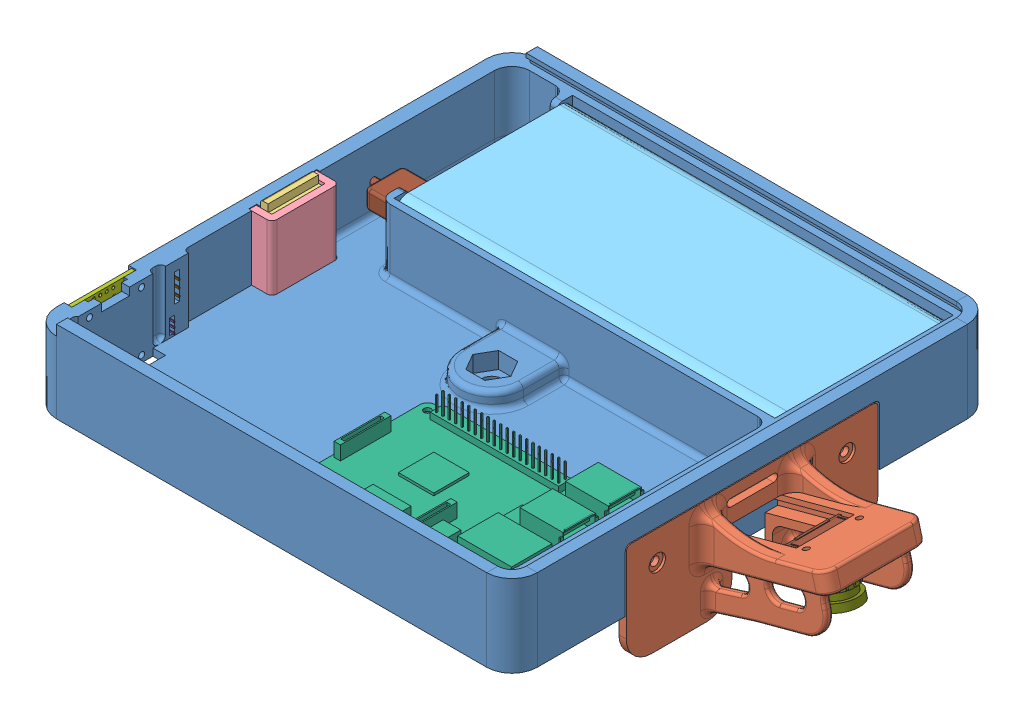
SolidWorks assembly vision, configuration Défaut. Lengths in mm.
Overall size (246.21 50.4 190).
58 component instances, 37 part files, 59 mates.
Components (placement in the parent):
- box-1: box [Défaut] at origin size (190.6 32.4 190)
- cover-1: cover [Défaut] at (-1.3 28.3 0) x (0 0 1) z (-1 0 0) size (190 2 187) (hidden)
- LogoARIG2-1: LogoARIG2 [Défaut] at (29.3179 30.3 42.8) x (0 0 -1) z (0 1 0) size (88.08 45.8 6.03) (hidden)
- support-cam-1: support-cam [Défaut] at (92 2.85 0) x (0 0 -1) z (1 0 0) size (99.5 41.7 53.04)
- latch-1: latch [Défaut] at (-84.4 7.063 -10) size (14.06 23.3 20)
- latch-box-1: latch-box [Défaut] at (-81.6 1.6 0) x (0 0 -1) z (1 0 0) size (26.6 26.5 9)
- Xiaomi PowerBank-1: Xiaomi PowerBank [Défaut] at (84.75 2.8 -89.15) x (0 0 1) z (-1 0 0) size (70 25 150)
- raspberryPi3BSimplified_STEP.step-1: raspberryPi3BSimplified_STEP.step [Défaut] at (32.5 6.8 51.4) x (1 0 0) z (0 1 0) size (87 58.5 18.55)
- OSSD-128x64.igs-1: OSSD-128x64.igs [Défaut] at (-91.9 15.3 69.5) x (0 0 1) z (0 -1 0) size (25 5.1 26)
- micro push button-2: micro push button [Défaut] at (-89.5 6.8667 45.1) x (0 -1 0) z (0 0 -1) size (5.8 13.4 5.8)
- mini swich-1: mini swich [Défaut] at (-89.9 19.2833 45.2) x (0 1 0) z (0 0 1) size (10.5 12.4 5.6)
- spring-1: spring [Défaut] at (-87.002 2.3106 6.0058) x (0.974863 -0.040201 -0.21915) z (0.219381 0.001367 0.975638) size (4.02 10.6 4.01)
- spring-2: spring [Défaut] at (-87.0662 11.9402 -5.894) x (-0.826432 0.000175 -0.563036) z (-0.56297 -0.015546 0.826331) size (4.02 10.6 4.01)
- usb-port-1: usb-port [Défaut] at (-65.85 15.3 -33.65) x (0 0 1) z (-1 0 0) size (15.2 7.3 34.7)
- RspCameraMia-1: RspCameraMia [Défaut] at (130.1784 16.2188 -0.0942) x (0.965926 0.258819 0) z (0.258819 -0.965926 0) size (23.86 25 22.7)
  - RspCameraMia.stp-1: RspCameraMia.stp [Défaut] at origin size (23.86 25 9.96)
    - 70521906.stp-1: 70521906.stp [Défaut] at (1.7167 0.8597 0.0159) size (2 2.1 0.95)
      - 70521906_01.stp-1: 70521906_01.stp [Défaut] at origin size (0.25 0.55 0.75)
      - 70521906_02.stp-1: 70521906_02.stp [Défaut] at origin size (0.25 0.55 0.75)
      - 70521906_03.stp-1: 70521906_03.stp [Défaut] at origin size (2 1.25 0.9)
      - 70521906_04.stp-1: 70521906_04.stp [Défaut] at origin size (0.25 0.55 0.75)
      - 70521906_05.stp-1: 70521906_05.stp [Défaut] at origin size (0.25 0.55 0.75)
      - 70521906_06.stp-1: 70521906_06.stp [Défaut] at origin size (0.25 0.55 0.75)
      - 70521906_07.stp-1: 70521906_07.stp [Défaut] at origin size (0.25 0.55 0.75)
    - PicameraPCB.stp-1: PicameraPCB.stp [Défaut] at (0.2393 -0.0199 0) x (-1 0 0) z (0 0 1) size (23.86 25 2.2)
    - OVA5647_Housing.stp-1: OVA5647_Housing.stp [Défaut] at (-2.4078 0.0859 1) x (1 0 0) z (0 -1 0) size (8 3.95 8)
    - OVA5647_Lens_FOV.stp-1: OVA5647_Lens_FOV.stp [Défaut] at (-2.4087 0.0921 5.963) x (1 0 0) z (0 -1 0) size (6 3.35 6)
    - ribbon_cam.stp-1: ribbon_cam.stp [Défaut] at (-2.4804 0.3633 1.4162) x (0 1 0) z (1 0 0) size (5.6 0.69 4.76)
    - CCD.stp-1: CCD.stp [Défaut] at (-2.0757 0.287 1.296) x (1 0 0) z (0 -1 0) size (8.01 0.69 8.01)
    - CAPC-0805-T0.75-BN.stp-1: CAPC-0805-T0.75-BN.stp [Défaut] at (4.562 5.9833 -0.0026) x (0 -1 0) z (0 0 -1) size (2.1 1.35 0.75)
    - CAPC-0805-T0.75-BN.stp-2: CAPC-0805-T0.75-BN.stp [Défaut] at (2.0233 10.2705 -0.0026) x (0 -1 0) z (0 0 -1) size (2.1 1.35 0.75)
    - CAPC-0402-T0.55-BN.stp-1: CAPC-0402-T0.55-BN.stp [Défaut] at (-2.9562 6.224 -0.2572) x (-1 0 0) z (0 -1 0) size (1.05 0.55 0.55)
    - CAPC-0402-T0.55-BN.stp-2: CAPC-0402-T0.55-BN.stp [Défaut] at (-2.9504 5.2898 -0.2691) x (-1 0 0) z (0 -1 0) size (1.05 0.55 0.55)
    - CAPC-0402-T0.55-BN.stp-3: CAPC-0402-T0.55-BN.stp [Défaut] at (4.5768 -5.1833 -0.2811) x (-1 0 0) z (0 -1 0) size (1.05 0.55 0.55)
    - CAPC-0402-T0.55-BN.stp-4: CAPC-0402-T0.55-BN.stp [Défaut] at (2.5547 -5.1368 -0.2811) x (-1 0 0) z (0 -1 0) size (1.05 0.55 0.55)
    - CAPC-0402-T0.55-BN.stp-5: CAPC-0402-T0.55-BN.stp [Défaut] at (2.6129 -9.93 -0.293) x (-1 0 0) z (0 -1 0) size (1.05 0.55 0.55)
    - CAPC-0402-T0.55-BN.stp-6: CAPC-0402-T0.55-BN.stp [Défaut] at (4.7286 -9.9294 -0.293) x (-1 0 0) z (0 -1 0) size (1.05 0.55 0.55)
    - CAPC-0402-T0.55-BN.stp-7: CAPC-0402-T0.55-BN.stp [Défaut] at (8.4068 -3.8793 -0.2811) x (-1 0 0) z (0 -1 0) size (1.05 0.55 0.55)
    - CAPC-0402-T0.55-BN.stp-8: CAPC-0402-T0.55-BN.stp [Défaut] at (9.0088 0.0217 -0.2796) x (0 1 0) z (-1 0 0) size (1.05 0.55 0.55)
    - CAPC-0402-T0.55-BN.stp-9: CAPC-0402-T0.55-BN.stp [Défaut] at (10.4284 2.6731 -0.3022) x (0 1 0) z (-1 0 0) size (1.05 0.55 0.55)
    - CAPC-0402-T0.55-BN.stp-10: CAPC-0402-T0.55-BN.stp [Défaut] at (8.2321 1.3259 -0.2838) x (1 0 0) z (0 1 0) size (1.05 0.55 0.55)
    - RESC-0402.stp-1: RESC-0402.stp [Défaut] at (3.7919 0.0148 -0.0114) x (1 0 0) z (0 0 -1) size (1.05 0.55 0.4)
    - RESC-0402.stp-2: RESC-0402.stp [Défaut] at (4.1232 2.6296 -0.0028) x (0 -1 0) z (0 0 -1) size (1.05 0.55 0.4)
    - RESC-0402.stp-3: RESC-0402.stp [Défaut] at (10.5883 -6.2795 -0.0019) x (0 1 0) z (0 0 -1) size (1.05 0.55 0.4)
    - RESC-0603.stp-1: RESC-0603.stp [Défaut] at (-2.6191 7.0617 -0.0121) x (1 0 0) z (0 0 -1) size (1.7 0.9 0.55)
    - RESC-0603.stp-2: RESC-0603.stp [Défaut] at (-3.4466 3.0018 -0.0048) x (0 -1 0) z (0 0 -1) size (1.7 0.9 0.55)
    - RESC-1210.stp-1: RESC-1210.stp [Défaut] at (2.2265 5.9002 -0.0068) x (0 -1 0) z (0 0 -1) size (3.3 2.7 0.6)
    - c-1-1734248-5-e-raspberry_display.stp-1: c-1-1734248-5-e-raspberry_display.stp [Défaut] at (-10.6651 0.0449 -1.5) x (0 -1 0) z (-1 0 0) size (22.4 3.22 5.68)
    - SOT23-5.stp-1: SOT23-5.stp [Défaut] at (4.2989 9.8879 0.5457) x (0 -1 0) z (0 0 -1) size (2.84 3.03 1.19)
    - SOT23-5.stp-2: SOT23-5.stp [Défaut] at (3.5194 -3.2493 0.04) x (-1 0 0) z (0 0 -1) size (2.84 3.03 1.19)
    - SOT23-5.stp-3: SOT23-5.stp [Défaut] at (3.5816 -8.055 0.0206) x (-1 0 0) z (0 0 -1) size (2.84 3.03 1.19)
    - KX7 SMD Quartz Crystal Resonator 3.2x2.5mm.stp-1: KX7 SMD Quartz Crystal Resonator 3.2x2.5mm.stp [Défaut] at (9.9746 -4.9221 0.0339) x (-1 0 0) z (0 -1 0) size (3.2 0.6 2.5)
    - c6aaa.stp-1: c6aaa.stp [Défaut] at (0.0643 0.0942 0) x (1 0 0) z (0 0 -1) size (2 2.99 0.6)
    - 4pin_smd.stp-1: 4pin_smd.stp [Défaut] at (0.027 0.0676 0) x (1 0 0) z (0 0 -1) size (1.29 1 0.47)
    - 4pin_smd.stp-2: 4pin_smd.stp [Défaut] at (-0.0093 -6.0092 -0.0198) x (1 0 0) z (0 0 -1) size (1.29 1 0.47)
    - 4pin_smd.stp-3: 4pin_smd.stp [Défaut] at (0.0326 -3.0068 -0.0235) x (1 0 0) z (0 0 -1) size (1.29 1 0.47)
  - WideAngleLens.step-1: WideAngleLens.step [Défaut] at (-4.3167 0.0942 2.6) x (1 0 0) z (0 -1 0) size (14 16.9 14)
- central-nut-1: central-nut [Défaut] at (-8 2.8 0) x (0 0 -1) z (1 0 0) size (34 10.5 36) (hidden)
Mates (geometry in assembly coordinates):
- Largeur1: width: plane of Xiaomi PowerBank-1 through (-65.25 2.8 -89.15) normal (0 0 -1); plane of Xiaomi PowerBank-1 through (-65.25 2.8 -19.15) normal (0 0 1); plane of box-1 through (-95 28.3 -89.4) normal (0 0 1); plane of box-1 through (0 198.2229 -18.9) normal (0 0 -1)
- Coïncidente1: coincident: plane of box-1 through (0 2.8 0) normal (0 1 0); plane of Xiaomi PowerBank-1 through (-65.25 2.8 -89.15) normal (0 -1 0)
- Largeur2: width: plane of Xiaomi PowerBank-1 through (84.75 2.8 -89.15) normal (1 0 0); plane of Xiaomi PowerBank-1 through (-65.25 2.8 -89.15) normal (-1 0 0); plane of box-1 through (-65.5 198.2229 0) normal (1 0 0); plane of box-1 through (85 28.3 -95) normal (-1 0 0)
- Coïncidente8: coincident: plane of box-1 through (0 28.3 0) normal (0 1 0); plane of cover-1 through (-1.3 28.3 0) normal (0 -1 0)
- Largeur3: width: plane of cover-1 through (92.2 30.3 -92) normal (0 0 -1); plane of cover-1 through (92.2 30.3 92) normal (0 0 1); plane of box-1 through (-85 30.8 92.2) normal (0 0 -1); plane of box-1 through (85 30.8 -92.2) normal (0 0 1)
- Tangent3: tangent: face of OSSD-128x64.igs-1; plane of box-1 through (-91.9 0 0) normal (-1 0 0)
- Coïncidente10: coincident: plane of box-1 through (51.5 6.8 75.9) normal (0 1 0); plane of ? through (-6.225 6.8 27.125) normal (0 -1 0)
- Coaxiale1: concentric: circle of ?; cylinder of box-1 through (-6.5 6.8 49.9) axis (0 1 0) radius 2
- Parallèle3: parallel: plane of box-1 through (-95 28.3 89.4) normal (0 0 -1); plane of ? through (-6.225 8.3 23.375) normal (0 0 -1)
- Coïncidente12: coincident: plane of box-1 through (51.5 6.8 26.9) normal (0 1 0); plane of raspberryPi3BSimplified_STEP.step-1 through (32.5 6.8 51.4) normal (0 -1 0)
- Coaxiale4: concentric: cylinder of raspberryPi3BSimplified_STEP.step-1 through (51.5 6.8 26.9) axis (0 1 0) radius 1.375; cylinder of box-1 through (51.5 6.8 26.9) axis (0 1 0) radius 2
- Parallèle4: parallel: plane of box-1 through (-95 28.3 89.4) normal (0 0 -1); plane of raspberryPi3BSimplified_STEP.step-1 through (-10 8.1 23.4) normal (0 0 -1)
- Coïncidente14: coincident: plane of box-1 through (-129.3376 -3.6169 174.3263) normal (-1 0 0); plane of ? through (-129.3376 17.3498 214.3583) normal (1 0 0)
- Coïncidente15: coincident: plane of box-1 through (-129.3376 20.2498 217.2583) normal (0 0 -1); plane of ? through (-134.6376 20.2498 217.2583) normal (0 0 1)
- Coïncidente16: coincident: plane of box-1 through (-129.3376 20.2498 217.2583) normal (0 -1 0); plane of ? through (-134.6376 20.2498 217.2583) normal (0 1 0)
- Coïncidente17: coincident: plane of box-1 through (-89.5 0 0) normal (-1 0 0); plane of micro push button-2 through (-89.5 6.8667 45.1) normal (1 0 0)
- Coïncidente18: coincident: plane of box-1 through (-89.5 9.7667 48) normal (0 0 -1); plane of micro push button-2 through (-94.8 9.7667 48) normal (0 0 1)
- Coïncidente19: coincident: plane of box-1 through (-89.5 9.7667 48) normal (0 -1 0); plane of micro push button-2 through (-94.8 9.7667 48) normal (0 1 0)
- Coïncidente20: coincident: plane of box-1 through (-89.4 28.3 -95) normal (1 0 0); plane of latch-1 through (-89.4 23.063 10) normal (-1 0 0)
- Largeur7: width: plane of box-1 through (95.001 23.3 10.25) normal (0 0 -1); plane of box-1 through (95.001 23.3 -10.25) normal (0 0 1); plane of latch-1 through (-84.4 7.063 10) normal (0 0 1); plane of latch-1 through (-84.4 7.063 -10) normal (0 0 -1)
- DistanceLimite1: limit distance = 0.237 mm: plane of latch-1 through (-89.4 23.063 10) normal (0 1 0); plane of box-1 through (95.001 23.3 -10.25) normal (0 -1 0)
- DistanceLimite2: limit distance = 3.263 mm: plane of box-1 through (95.001 10.8 -10.25) normal (0 1 0); plane of latch-1 through (-95 14.063 10) normal (0 -1 0)
- Coïncidente24: coincident: plane of box-1 through (0 1.6 0) normal (0 1 0); plane of latch-box-1 through (-81.6 1.6 0) normal (0 -1 0)
- Coïncidente25: coincident: plane of box-1 through (-90.6 -28.0297 13.45) normal (1 0 0); plane of latch-box-1 through (-90.6 28.1 10.5) normal (-1 0 0)
- Largeur8: width: plane of latch-box-1 through (-90.6 28.1 -10.5) normal (0 0 1); plane of latch-box-1 through (-84.4 28.1 10.5) normal (0 0 -1); plane of box-1 through (95.001 23.3 -10.25) normal (0 0 1); plane of box-1 through (95.001 23.3 10.25) normal (0 0 -1)
- Coïncidente26: coincident: plane of box-1 through (92 0 0) normal (1 0 0); plane of support-cam-1 through (92 2.85 0) normal (-1 0 0)
- Largeur9: width: plane of support-cam-1 through (94.9 23.7 -49.75) normal (0 0 -1); plane of support-cam-1 through (94.9 23.7 49.75) normal (0 0 1); plane of box-1 through (92 0 -50.25) normal (0 0 1); plane of box-1 through (92 0 50.25) normal (0 0 -1)
- Largeur10: width: plane of ? through (117.0821 9.879 0) normal (-0.087156 0.996195 0); plane of ? through (117.1605 8.9825 0) normal (0.087156 -0.996195 0); plane of support-cam-1; plane of support-cam-1
- Largeur11: width: plane of ? through (131.5269 11.1428 12.5) normal (0 0 1); plane of ? through (131.5269 11.1428 -12.5) normal (0 0 -1); plane of support-cam-1 through (90.1136 5.5621 13) normal (0 0 -1); plane of support-cam-1 through (90.1136 5.5621 -13) normal (0 0 1)
- Coaxiale5: concentric: circle of support-cam-1; circle of ?
- Coïncidente28: coincident: plane of box-1 through (-89.9 0 0) normal (-1 0 0); plane of mini swich-1 through (-89.9 19.2833 45.2) normal (1 0 0)
- Coïncidente29: coincident: plane of box-1 through (-89.9 0 48) normal (0 0 -1); plane of mini swich-1 through (-94.8 14.0333 48) normal (0 0 1)
- Coïncidente30: coincident: plane of box-1 through (-89.9 24.5333 0) normal (0 -1 0); plane of mini swich-1 through (-94.8 24.5333 42.4) normal (0 1 0)
- Coaxiale7: concentric: cylinder of box-1 through (95.001 7.075 48.5) axis (-1 0 0) radius 2.6; cone of ? through (-91.9998 7.075 48.5) axis (-1 0 0)
- Coïncidente32: coincident: plane of box-1 through (-89.4 28.3 -95) normal (1 0 0); plane of ? through (-89.4 7.075 48.5) normal (-1 0 0)
- Coïncidente34: coincident: plane of box-1 through (0 0 0) normal (0 0 1); plane of assembly through (0 0 0) normal (0 0 1)
- Coïncidente35: coincident: plane of box-1 through (0 0 0) normal (0 1 0); plane of assembly through (0 0 0) normal (0 1 0)
- Coïncidente36: coincident: plane of box-1 through (0 0 0) normal (1 0 0); plane of assembly through (0 0 0) normal (1 0 0)
- Tangent4: tangent: plane of latch-1 through (-86.9 12.063 6) normal (0 -1 0); face of spring-1
- Tangent5: tangent: cylinder of latch-1 through (-86.9 12.063 6) axis (0 -1 0) radius 2; face of spring-1
- Tangent6: tangent: plane of latch-1 through (-86.9 12.063 -6) normal (0 -1 0); face of spring-2
- Tangent7: tangent: cylinder of latch-1 through (-86.9 12.063 -6) axis (0 -1 0) radius 2; face of spring-2
- Coaxiale9: concentric: cylinder of box-1 through (92 12 37.5) axis (1 0 0) radius 2.1; cylinder of support-cam-1 through (94.9 12 37.5) axis (1 0 0) radius 1.7
- Coïncidente37: coincident: plane of Xiaomi PowerBank-1 through (-53.75 2.8 -89.15) normal (-1 0 0); plane of usb-port-1 through (-53.75 15.3 -33.65) normal (1 0 0)
- Largeur12: width: plane of usb-port-1 through (-53.75 17.55 -27.65) normal (0 1 0); plane of usb-port-1 through (-53.75 13.05 -27.65) normal (0 -1 0); plane of Xiaomi PowerBank-1 through (-53.75 18.8 -40.15) normal (0 -1 0); plane of Xiaomi PowerBank-1 through (-53.75 11.8 -40.15) normal (0 1 0)
- Largeur13: width: plane of Xiaomi PowerBank-1 through (-53.75 18.8 -40.15) normal (0 0 1); plane of Xiaomi PowerBank-1 through (-53.75 18.8 -27.15) normal (0 0 -1); plane of usb-port-1 through (-53.75 17.55 -39.65) normal (0 0 -1); plane of usb-port-1 through (-53.75 17.55 -27.65) normal (0 0 1)
- Tangent8: tangent: plane of box-1 through (-90.5 0 82) normal (0 0 -1); face of OSSD-128x64.igs-1
- Tangent9: tangent: plane of box-1 through (0 28.3 0) normal (0 1 0); face of OSSD-128x64.igs-1
- DistanceLimite3: limit distance = 0 mm: plane of box-1 through (92.2 30.8 85) normal (-1 0 0); plane of cover-1 through (92.2 30.3 -92) normal (1 0 0)
- Verrouiller1: lock: unknown of cover-1; unknown of LogoARIG2-1
- Largeur14: width: plane of ? through (115.5075 10.0926 0) normal (-0.087156 0.996195 0); plane of ? through (115.647 8.4987 0) normal (0.087156 -0.996195 0); plane of support-cam-1; plane of support-cam-1
- Largeur15: width: plane of ? through (131.6359 9.8975 -16.05) normal (0 0 -1); plane of ? through (99.658 7.0998 16.05) normal (0 0 1); plane of support-cam-1 through (90.1136 5.5621 -13) normal (0 0 1); plane of support-cam-1 through (90.1136 5.5621 13) normal (0 0 -1)
- Coïncidente38: coincident: plane of ? through (131.5269 11.1428 12.5) normal (0.996195 0.087156 0); plane of ? through (131.6359 9.8975 16.05) normal (0.996195 0.087156 0)
- Largeur16: width: plane of RspCameraMia-1/RspCameraMia.stp-1/PicameraPCB.stp-1 through (139.8331 18.8057 12.5) normal (0 0 1); plane of RspCameraMia-1/RspCameraMia.stp-1/PicameraPCB.stp-1 through (120.6479 13.6651 -12.5) normal (0 0 -1); plane of support-cam-1 through (86.2616 3.416 13) normal (0 0 -1); plane of support-cam-1 through (86.2616 3.416 -13) normal (0 0 1)
- Coïncidente39: coincident: plane of RspCameraMia-1/RspCameraMia.stp-1/PicameraPCB.stp-1 through (130.4993 15.2695 0) normal (0.258819 -0.965926 0); plane of support-cam-1 through (86.2616 3.416 13) normal (-0.258819 0.965926 0)
- Coaxiale10: concentric: cylinder of support-cam-1 through (123.3313 32.0952 -10.5) axis (0.258819 -0.965926 0) radius 1.2; cylinder of RspCameraMia-1/RspCameraMia.stp-1/PicameraPCB.stp-1 through (136.7231 -17.8838 -10.5) axis (0.258819 -0.965926 0) radius 1.1
- Coïncidente40: coincident: plane of box-1 through (0 2.8 0) normal (0 1 0); plane of central-nut-1 through (-8 2.8 0) normal (0 -1 0)
- Coaxiale11: concentric: cylinder of box-1 through (-8 28.3 0) axis (0 -1 0) radius 4; cylinder of central-nut-1 through (-8 13.3 0) axis (0 1 0) radius 4
- Parallèle5: parallel: plane of box-1 through (0 198.2229 -16.1) normal (0 0 1); plane of central-nut-1 through (-26 13.3 -16) normal (0 0 -1)
